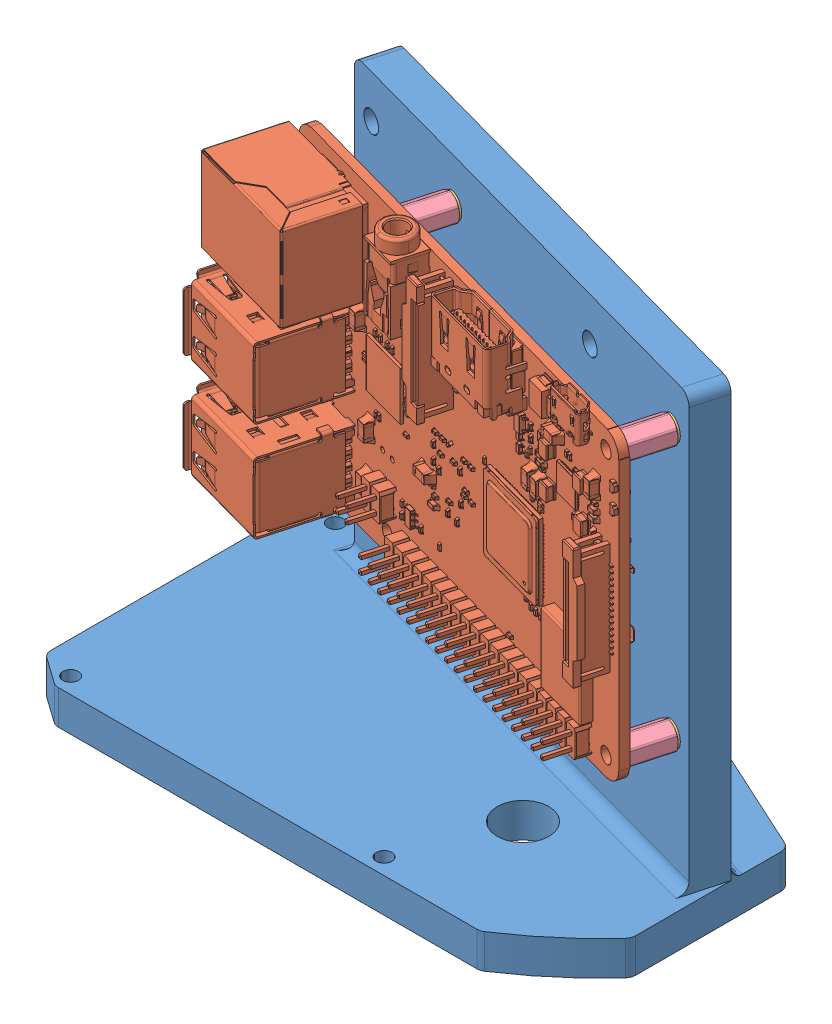
SolidWorks assembly Pi+Mount, configuration Default. Lengths in mm.
Overall size (99.85 86.35 55).
10 component instances, 4 part files, 22 mates.
Components (placement in the parent):
- Pi mount-1: Pi mount [Default] at origin size (99.85 86.35 55)
- raspberry_pi_3_b_plus-1: raspberry_pi_3_b_plus [Default] at (19.0827 53.85 -1.264) x (-0.963854 0 -0.266432) z (-0.266432 0 0.963854) size (87.29 58.46 20.03)
- 94180A321_M2.5 heat insert-4: 94180A321_M2.5 heat insert [94180A321] at (59.2614 78.35 -0.237) x (0.963854 0 0.266432) z (-0.266432 0 0.963854) size (4.37 4.37 3.43)
- 94180A321_M2.5 heat insert-9: 94180A321_M2.5 heat insert [94180A321] at (59.2614 29.35 -0.237) x (0.963854 0 0.266432) z (-0.266432 0 0.963854) size (4.37 4.37 3.43)
- 94180A321_M2.5 heat insert-10: 94180A321_M2.5 heat insert [94180A321] at (3.3578 29.35 -15.6901) x (0.963854 0 0.266432) z (-0.266432 0 0.963854) size (4.37 4.37 3.43)
- 94180A321_M2.5 heat insert-11: 94180A321_M2.5 heat insert [94180A321] at (3.3578 78.35 -15.6901) x (0.963854 0 0.266432) z (-0.266432 0 0.963854) size (4.37 4.37 3.43)
- 93655A094_M2.5 8mm M-F standoff-5: 93655A094_M2.5 8mm M-F standoff [93655A094] at (2.9009 29.35 -14.0371) x (0.963854 0 0.266432) z (-0.266432 0 0.963854) size (4.5 5.08 12.09)
- 93655A094_M2.5 8mm M-F standoff-6: 93655A094_M2.5 8mm M-F standoff [93655A094] at (2.9009 78.35 -14.0371) x (0.963854 0 0.266432) z (-0.266432 0 0.963854) size (4.5 5.08 12.09)
- 93655A094_M2.5 8mm M-F standoff-7: 93655A094_M2.5 8mm M-F standoff [93655A094] at (58.8044 29.35 1.416) x (0.963854 0 0.266432) z (-0.266432 0 0.963854) size (4.5 5.08 12.09)
- 93655A094_M2.5 8mm M-F standoff-8: 93655A094_M2.5 8mm M-F standoff [93655A094] at (58.8044 78.35 1.416) x (0.963854 0 0.266432) z (-0.266432 0 0.963854) size (4.5 5.08 12.09)
Mates (geometry in assembly coordinates):
- Coincident2: coincident aligned: plane of Pi mount-1 through (0 0 0) normal (1 0 0)
- Coincident5: coincident aligned: plane of Pi mount-1 through (0 0 0) normal (0 0 1)
- Coincident6: coincident aligned: plane of Pi mount-1 through (0 0 0) normal (0 1 0)
- Concentric82: concentric aligned: cylinder of 94180A321_M2.5 heat insert-4 through (58.8044 78.35 1.416) axis (-0.266432 0 0.963854) radius 1.25; cylinder of Pi mount-1 through (58.8958 78.35 1.0854) axis (-0.266432 0 0.963854) radius 1.9304
- Coincident223: coincident anti-aligned: plane of Pi mount-1 through (-22.3741 86.35 -21.3795) normal (-0.266432 0 0.963854); plane of 94180A321_M2.5 heat insert-4 through (58.8958 80.535 1.0854) normal (0.266432 0 -0.963854)
- Concentric83: concentric aligned: cylinder of 94180A321_M2.5 heat insert-11 through (2.9009 78.35 -14.0371) axis (-0.266432 0 0.963854) radius 1.25; cylinder of Pi mount-1 through (2.9923 78.35 -14.3677) axis (-0.266432 0 0.963854) radius 1.9304
- Coincident224: coincident anti-aligned: plane of Pi mount-1 through (-22.3741 86.35 -21.3795) normal (-0.266432 0 0.963854); plane of 94180A321_M2.5 heat insert-11 through (2.9923 80.535 -14.3677) normal (0.266432 0 -0.963854)
- Concentric84: concentric aligned: cylinder of Pi mount-1 through (2.9923 29.35 -14.3677) axis (-0.266432 0 0.963854) radius 1.9304; cylinder of 94180A321_M2.5 heat insert-10 through (2.9009 29.35 -14.0371) axis (-0.266432 0 0.963854) radius 1.25
- Coincident225: coincident anti-aligned: plane of Pi mount-1 through (-22.3741 86.35 -21.3795) normal (-0.266432 0 0.963854); plane of 94180A321_M2.5 heat insert-10 through (2.9923 31.535 -14.3677) normal (0.266432 0 -0.963854)
- Concentric85: concentric aligned: cylinder of Pi mount-1 through (58.8958 29.35 1.0854) axis (-0.266432 0 0.963854) radius 1.9304; cylinder of 94180A321_M2.5 heat insert-9 through (58.8044 29.35 1.416) axis (-0.266432 0 0.963854) radius 1.25
- Coincident226: coincident anti-aligned: plane of Pi mount-1 through (-22.3741 86.35 -21.3795) normal (-0.266432 0 0.963854); plane of 94180A321_M2.5 heat insert-9 through (58.8958 31.535 1.0854) normal (0.266432 0 -0.963854)
- Concentric89: concentric anti-aligned: cylinder of 94180A321_M2.5 heat insert-4 through (58.8044 78.35 1.416) axis (-0.266432 0 0.963854) radius 1.25; cylinder of 93655A094_M2.5 8mm M-F standoff-8 through (59.8435 78.35 -2.343) axis (0.266432 0 -0.963854) radius 0.9577
- Coincident227: coincident anti-aligned: plane of 94180A321_M2.5 heat insert-4 through (58.8044 79.6 1.416) normal (-0.266432 0 0.963854); plane of 93655A094_M2.5 8mm M-F standoff-8 through (58.8044 79.5327 1.416) normal (0.266432 0 -0.963854)
- Concentric90: concentric anti-aligned: cylinder of 94180A321_M2.5 heat insert-11 through (2.9009 78.35 -14.0371) axis (-0.266432 0 0.963854) radius 1.25; cylinder of 93655A094_M2.5 8mm M-F standoff-6 through (3.94 78.35 -17.7961) axis (0.266432 0 -0.963854) radius 0.9577
- Coincident228: coincident anti-aligned: plane of 94180A321_M2.5 heat insert-11 through (2.9009 79.6 -14.0371) normal (-0.266432 0 0.963854); plane of 93655A094_M2.5 8mm M-F standoff-6 through (2.9009 79.5327 -14.0371) normal (0.266432 0 -0.963854)
- Concentric91: concentric anti-aligned: cylinder of 94180A321_M2.5 heat insert-9 through (58.8044 29.35 1.416) axis (-0.266432 0 0.963854) radius 1.25; cylinder of 93655A094_M2.5 8mm M-F standoff-7 through (59.8435 29.35 -2.343) axis (0.266432 0 -0.963854) radius 0.9577
- Coincident229: coincident anti-aligned: plane of 94180A321_M2.5 heat insert-9 through (58.8044 30.6 1.416) normal (-0.266432 0 0.963854); plane of 93655A094_M2.5 8mm M-F standoff-7 through (58.8044 30.5327 1.416) normal (0.266432 0 -0.963854)
- Concentric92: concentric anti-aligned: cylinder of 94180A321_M2.5 heat insert-10 through (2.9009 29.35 -14.0371) axis (-0.266432 0 0.963854) radius 1.25; cylinder of 93655A094_M2.5 8mm M-F standoff-5 through (3.94 29.35 -17.7961) axis (0.266432 0 -0.963854) radius 0.9577
- Coincident230: coincident anti-aligned: plane of 94180A321_M2.5 heat insert-10 through (2.9009 30.6 -14.0371) normal (-0.266432 0 0.963854); plane of 93655A094_M2.5 8mm M-F standoff-5 through (2.9009 30.5327 -14.0371) normal (0.266432 0 -0.963854)
- Concentric101: concentric aligned: cylinder of Pi mount-1 through (58.8958 29.35 1.0854) axis (-0.266432 0 0.963854) radius 1.9304; cylinder of raspberry_pi_3_b_plus-1 through (56.673 29.35 9.1268) axis (-0.266432 0 0.963854) radius 1.375
- Concentric102: concentric aligned: cylinder of Pi mount-1 through (2.9923 78.35 -14.3677) axis (-0.266432 0 0.963854) radius 1.9304; cylinder of raspberry_pi_3_b_plus-1 through (0.7695 78.35 -6.3262) axis (-0.266432 0 0.963854) radius 1.375
- Coincident231: coincident anti-aligned: plane of raspberry_pi_3_b_plus-1 through (19.0827 53.85 -1.264) normal (0.266432 0 -0.963854); plane of 93655A094_M2.5 8mm M-F standoff-6 through (0.7695 79.825 -6.3262) normal (-0.266432 0 0.963854)
